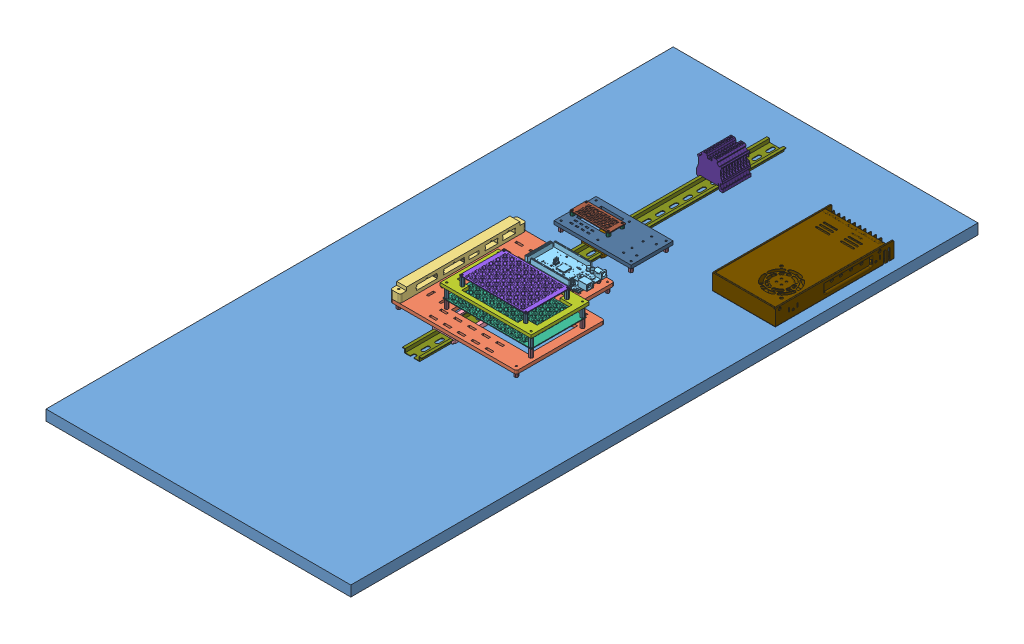
SolidWorks assembly Integrated Stand Base, configuration Default. Lengths in mm.
Overall size (552.45 92.11 1136.74).
89 component instances, 18 part files, 7 mates.
Components (placement in the parent):
- Base Stand-1: Base Stand [Default] at origin size (552.45 19.05 1136.74)
- Final_Assembly-1: Final_Assembly [Default] at (-199.0521 -63.7075 69.9554) x (0 0 -1) z (1 0 0) size (660.4 81.74 228.6)
  - Main board-1: Main board [Default] at (85.8748 92.7975 191.1146) size (228.6 6.1 228.6)
  - Connector_Holder-1: Connector_Holder [Default] at (-28.4252 98.8935 94.5946) size (228.6 20.32 17.78)
  - Main board din_rail-1: Main board din_rail [Default] at (200.1748 82.6375 173.6146) x (0 0 1) z (-1 0 0) size (40.89 10.16 228.6)
  - arduinoMega-1: arduinoMega [Detailed] at (160.8248 113.9303 205.0746) x (0 0 -1) z (1 0 0) size (108.32 14.5 53.3)
  - Flipper board-1: Flipper board [Default] at (53.4898 115.2003 220.1722) x (0 0 -1) z (-1 0 0) size (160.02 1.27 99.82)
  - LED_mount-1: LED_mount [Default] at (53.3628 133.7169 220.4262) x (0 0 -1) z (1 0 0) size (165.1 5.59 105.16)
  - LED_control_board-1: LED_control_board [Default] at (53.999 155.8149 220.1956) x (-0.002965 0 0.999996) z (0.999996 0 0.002965) size (120 1.47 80)
  - Output board din rail-1: Output board din rail [Default] at (241.4498 82.6375 173.6146) x (0 0 -1) z (1 0 0) size (40.89 10.16 76.2)
  - Output board-1: Output board [Default] at (317.6498 92.7975 243.4646) x (0 0 -1) z (1 0 0) size (139.7 6.1 76.2)
  - Output_Board-1: Output_Board [Default] at (279.9067 104.9133 144.6875) x (0 0 -1) z (1 0 0) size (71 1.47 30)
  - Spacer_Nut-3: Spacer_Nut [Default] at (6.8808 92.9245 296.8802) x (0 0 -1) z (0 1 0) size (6.48 5.61 2.41)
  - Spacer_Nut-5: Spacer_Nut [Default] at (6.8808 92.9245 143.769) x (0 0 -1) z (0 1 0) size (6.48 5.61 2.41)
  - Spacer_Nut-9: Spacer_Nut [Default] at (136.6748 92.9245 164.4446) x (0 0 -1) z (0 1 0) size (6.48 5.61 2.41)
  - Spacer_Nut-10: Spacer_Nut [Default] at (99.8448 92.9245 143.769) x (0 0 -1) z (0 1 0) size (6.48 5.61 2.41)
  - Spacer_Nut-12: Spacer_Nut [Default] at (136.6748 92.9245 239.1206) x (0.866025 0 -0.5) z (0 1 0) size (6.48 5.61 2.41)
  - Spacer_Nut-13: Spacer_Nut [Default] at (99.8448 92.9245 296.8802) x (0 0 -1) z (0 1 0) size (6.48 5.61 2.41)
  - Spacer_Nut-14: Spacer_Nut [Default] at (184.9348 92.9245 240.6446) x (0 0 -1) z (0 1 0) size (6.48 5.61 2.41)
  - Spacer_Nut-15: Spacer_Nut [Default] at (184.9348 92.9245 158.0946) x (0 0 -1) z (0 1 0) size (6.48 5.61 2.41)
  - Spacer_.592-1: Spacer_.592 [Default] at (6.8808 98.8935 143.769) x (0.866025 0 -0.5) z (0.5 0 0.866025) size (6.48 21.26 5.61)
  - Spacer_.592-2: Spacer_.592 [Default] at (6.8808 98.8935 296.8802) x (0 0 1) z (-1 0 0) size (6.48 21.26 5.61)
  - Spacer_.592-3: Spacer_.592 [Default] at (99.8448 98.8935 296.8802) x (0.866025 0 -0.5) z (0.5 0 0.866025) size (6.48 21.26 5.61)
  - Spacer_.592-4: Spacer_.592 [Default] at (99.8448 98.8935 143.769) x (0.866025 0 0.5) z (-0.5 0 0.866025) size (6.48 21.26 5.61)
  - Spacer_.592-5: Spacer_.592 [Default] at (136.6748 98.8935 164.4446) x (0.866025 0 -0.5) z (0.5 0 0.866025) size (6.48 21.26 5.61)
  - Spacer_.592-6: Spacer_.592 [Default] at (136.6748 98.8935 239.1206) x (0.866025 0 -0.5) z (0.5 0 0.866025) size (6.48 21.26 5.61)
  - Spacer_.592-7: Spacer_.592 [Default] at (184.9348 98.8935 240.6446) x (0.866025 0 -0.5) z (0.5 0 0.866025) size (6.48 21.26 5.61)
  - Spacer_.592-8: Spacer_.592 [Default] at (184.9348 98.8935 158.0946) x (0.866025 0 -0.5) z (0.5 0 0.866025) size (6.48 21.26 5.61)
  - Spacer_.778-6: Spacer_.778 [Default] at (6.8808 115.2003 296.8802) x (0.866025 0 0.5) z (-0.5 0 0.866025) size (6.48 21.26 5.61)
  - Spacer_.778-7: Spacer_.778 [Default] at (6.8808 115.2003 143.769) x (0 0 1) z (-1 0 0) size (6.48 21.26 5.61)
  - Spacer_.778-8: Spacer_.778 [Default] at (99.8448 115.2003 143.769) x (0.866025 0 0.5) z (-0.5 0 0.866025) size (6.48 21.26 5.61)
  - Spacer_.778-9: Spacer_.778 [Default] at (99.8448 115.2003 296.8802) x (0.866025 0 0.5) z (-0.5 0 0.866025) size (6.48 21.26 5.61)
  - Spacer_..237-2: Spacer_..237 [Default] at (6.8808 130.2371 296.8802) x (0.866025 0 -0.5) z (0.5 0 0.866025) size (6.48 12.24 5.61)
  - Spacer_..237-3: Spacer_..237 [Default] at (99.8448 130.2371 296.8802) x (0.866025 0 0.5) z (-0.5 0 0.866025) size (6.48 12.24 5.61)
  - Spacer_..237-4: Spacer_..237 [Default] at (6.8808 130.2371 143.769) x (0.866025 0 -0.5) z (0.5 0 0.866025) size (6.48 12.24 5.61)
  - Spacer_..237-5: Spacer_..237 [Default] at (99.8448 130.2371 143.769) x (0.866025 0 0.5) z (-0.5 0 0.866025) size (6.48 12.24 5.61)
  - Spacer_Nut-17: Spacer_Nut [Default] at (16.0248 133.8439 277.8862) x (0 0 -1) z (0 1 0) size (6.48 5.61 2.41)
  - Spacer_Nut-18: Spacer_Nut [Default] at (90.7008 133.8439 277.8862) x (-0.866025 0 -0.5) z (0 1 0) size (6.48 5.61 2.41)
  - Spacer_Nut-19: Spacer_Nut [Default] at (90.7008 133.8439 162.9662) x (0 0 -1) z (0 1 0) size (6.48 5.61 2.41)
  - Spacer_Nut-20: Spacer_Nut [Default] at (16.0248 133.8439 162.9662) x (-0.866025 0 0.5) z (0 1 0) size (6.48 5.61 2.41)
  - Spacer_.778-10: Spacer_.778 [Default] at (90.7008 139.3049 277.8862) x (0 0 1) z (-1 0 0) size (6.48 21.26 5.61)
  - Spacer_.778-11: Spacer_.778 [Default] at (90.7008 139.3049 162.9662) x (0.866025 0 -0.5) z (0.5 0 0.866025) size (6.48 21.26 5.61)
  - Spacer_.778-12: Spacer_.778 [Default] at (16.0248 139.3049 277.8862) x (0.866025 0 0.5) z (-0.5 0 0.866025) size (6.48 21.26 5.61)
  - Spacer_.778-13: Spacer_.778 [Default] at (16.0248 139.3049 162.9662) x (0.866025 0 -0.5) z (0.5 0 0.866025) size (6.48 21.26 5.61)
  - Spacer_..237-6: Spacer_..237 [Default] at (267.1038 98.8935 176.6626) x (0.5 0 0.866025) z (-0.866025 0 0.5) size (6.48 12.24 5.61)
  - 1.00m DIN Rail-1: 1.00m DIN Rail [26" LNG] at (414.4248 82.7575 173.6146) size (660.4 7.5 35)
  - Terminal Block Assembly-1: Terminal Block Assembly [Default] at (453.4648 83.4075 197.6146) x (1 0 0) z (0 1 0) size (51.51 55.11 56.59)
    - Terminal Block-2: Terminal Block [Default] at origin size (5.15 55.11 56.59)
      - pxc_3045088_17_UT-2-5-BK_3D.stp-1: pxc_3045088_17_UT-2-5-BK_3D.stp [Default] at origin size (5.15 55.11 56.59)
        - UT_2.5_BK-select.stp-1: UT_2.5_BK-select.stp [Default] at (5.15 -7.1989 17.4678) x (0 0.992546 -0.121869) z (1 0 0) size (49.27 50.96 5.15)
    - Terminal Block-3: Terminal Block [Default] at (5.1511 0 0) size (5.15 55.11 56.59)
      - pxc_3045088_17_UT-2-5-BK_3D.stp-1: pxc_3045088_17_UT-2-5-BK_3D.stp [Default] at origin size (5.15 55.11 56.59)
        - UT_2.5_BK-select.stp-1: UT_2.5_BK-select.stp [Default] at (5.15 -7.1989 17.4678) x (0 0.992546 -0.121869) z (1 0 0) size (49.27 50.96 5.15)
    - Terminal Block-4: Terminal Block [Default] at (10.3022 0 0) size (5.15 55.11 56.59)
      - pxc_3045088_17_UT-2-5-BK_3D.stp-1: pxc_3045088_17_UT-2-5-BK_3D.stp [Default] at origin size (5.15 55.11 56.59)
        - UT_2.5_BK-select.stp-1: UT_2.5_BK-select.stp [Default] at (5.15 -7.1989 17.4678) x (0 0.992546 -0.121869) z (1 0 0) size (49.27 50.96 5.15)
    - Terminal Block-5: Terminal Block [Default] at (15.4534 0 0) size (5.15 55.11 56.59)
      - pxc_3045088_17_UT-2-5-BK_3D.stp-1: pxc_3045088_17_UT-2-5-BK_3D.stp [Default] at origin size (5.15 55.11 56.59)
        - UT_2.5_BK-select.stp-1: UT_2.5_BK-select.stp [Default] at (5.15 -7.1989 17.4678) x (0 0.992546 -0.121869) z (1 0 0) size (49.27 50.96 5.15)
    - Terminal Block-6: Terminal Block [Default] at (20.6045 0 0) size (5.15 55.11 56.59)
      - pxc_3045088_17_UT-2-5-BK_3D.stp-1: pxc_3045088_17_UT-2-5-BK_3D.stp [Default] at origin size (5.15 55.11 56.59)
        - UT_2.5_BK-select.stp-1: UT_2.5_BK-select.stp [Default] at (5.15 -7.1989 17.4678) x (0 0.992546 -0.121869) z (1 0 0) size (49.27 50.96 5.15)
    - Terminal Block-7: Terminal Block [Default] at (25.7556 0 0) size (5.15 55.11 56.59)
      - pxc_3045088_17_UT-2-5-BK_3D.stp-1: pxc_3045088_17_UT-2-5-BK_3D.stp [Default] at origin size (5.15 55.11 56.59)
        - UT_2.5_BK-select.stp-1: UT_2.5_BK-select.stp [Default] at (5.15 -7.1989 17.4678) x (0 0.992546 -0.121869) z (1 0 0) size (49.27 50.96 5.15)
    - Terminal Block-8: Terminal Block [Default] at (30.9067 0 0) size (5.15 55.11 56.59)
      - pxc_3045088_17_UT-2-5-BK_3D.stp-1: pxc_3045088_17_UT-2-5-BK_3D.stp [Default] at origin size (5.15 55.11 56.59)
        - UT_2.5_BK-select.stp-1: UT_2.5_BK-select.stp [Default] at (5.15 -7.1989 17.4678) x (0 0.992546 -0.121869) z (1 0 0) size (49.27 50.96 5.15)
    - Terminal Block-9: Terminal Block [Default] at (36.0578 0 0) size (5.15 55.11 56.59)
      - pxc_3045088_17_UT-2-5-BK_3D.stp-1: pxc_3045088_17_UT-2-5-BK_3D.stp [Default] at origin size (5.15 55.11 56.59)
        - UT_2.5_BK-select.stp-1: UT_2.5_BK-select.stp [Default] at (5.15 -7.1989 17.4678) x (0 0.992546 -0.121869) z (1 0 0) size (49.27 50.96 5.15)
    - Terminal Block-10: Terminal Block [Default] at (41.209 0 0) size (5.15 55.11 56.59)
      - pxc_3045088_17_UT-2-5-BK_3D.stp-1: pxc_3045088_17_UT-2-5-BK_3D.stp [Default] at origin size (5.15 55.11 56.59)
        - UT_2.5_BK-select.stp-1: UT_2.5_BK-select.stp [Default] at (5.15 -7.1989 17.4678) x (0 0.992546 -0.121869) z (1 0 0) size (49.27 50.96 5.15)
    - Terminal Block-11: Terminal Block [Default] at (46.3601 0 0) size (5.15 55.11 56.59)
      - pxc_3045088_17_UT-2-5-BK_3D.stp-1: pxc_3045088_17_UT-2-5-BK_3D.stp [Default] at origin size (5.15 55.11 56.59)
        - UT_2.5_BK-select.stp-1: UT_2.5_BK-select.stp [Default] at (5.15 -7.1989 17.4678) x (0 0.992546 -0.121869) z (1 0 0) size (49.27 50.96 5.15)
  - Spacer_..237-7: Spacer_..237 [Default] at (291.9958 98.8935 176.6626) x (0.5 0 0.866025) z (-0.866025 0 0.5) size (6.48 12.24 5.61)
  - Spacer_..237-8: Spacer_..237 [Default] at (291.9958 98.8935 111.3846) x (0.5 0 0.866025) z (-0.866025 0 0.5) size (6.48 12.24 5.61)
  - Spacer_..237-9: Spacer_..237 [Default] at (267.1038 98.8935 111.3846) x (0.5 0 0.866025) z (-0.866025 0 0.5) size (6.48 12.24 5.61)
  - Spacer_.592-9: Spacer_.592 [Default] at (-20.8052 80.3007 84.4346) x (0 0 -1) z (1 0 0) size (6.48 21.26 5.61)
  - Spacer_.592-10: Spacer_.592 [Default] at (-20.8052 80.3007 297.7946) x (0 0 -1) z (1 0 0) size (6.48 21.26 5.61)
  - Spacer_.592-11: Spacer_.592 [Default] at (192.5548 80.3007 84.4346) x (0 0 -1) z (1 0 0) size (6.48 21.26 5.61)
  - Spacer_.592-12: Spacer_.592 [Default] at (193.8248 80.3007 248.2646) x (0 0 -1) z (1 0 0) size (6.48 21.26 5.61)
  - Spacer_.592-13: Spacer_.592 [Default] at (247.7998 80.3007 237.1146) x (0 0 -1) z (1 0 0) size (6.48 21.26 5.61)
  - Spacer_.592-14: Spacer_.592 [Default] at (311.2998 80.3007 237.1146) x (0 0 -1) z (1 0 0) size (6.48 21.26 5.61)
  - Spacer_.592-15: Spacer_.592 [Default] at (247.7998 80.3007 110.1146) x (0 0 -1) z (1 0 0) size (6.48 21.26 5.61)
  - Spacer_.592-16: Spacer_.592 [Default] at (311.2998 80.3007 110.1146) x (0 0 -1) z (1 0 0) size (6.48 21.26 5.61)
- Meanwell LRS-350-48 AC-DC Converter-1: Meanwell LRS-350-48 AC-DC Converter [Default] at (257.175 19.05 -220.0195) x (0 0 1) z (-1 0 0) size (215.21 30.1 114.01)
Mates (geometry in assembly coordinates):
- Parallel1: parallel aligned: plane of Base Stand-1 through (-276.225 19.05 568.3695) normal (0 0 1); plane of Final_Assembly-1/Main board-1 through (-122.2375 35.186 98.3805) normal (0 0 1)
- Distance1: distance = 153.9875 mm aligned: plane of Final_Assembly-1/Connector_Holder-1 through (-122.2375 35.186 98.3805) normal (-1 0 0); plane of Base Stand-1 through (-276.225 19.05 568.3695) normal (-1 0 0)
- Distance2: distance = 63.5 mm aligned: plane of Final_Assembly-1/1.00m DIN Rail-1 through (-7.9375 19.05 -504.8695) normal (0 0 -1); plane of Base Stand-1 through (-276.225 19.05 -568.3695) normal (0 0 -1)
- Coincident5: coincident anti-aligned: plane of Base Stand-1 through (0 19.05 0) normal (0 1 0); plane of Final_Assembly-1/1.00m DIN Rail-1 through (-7.9375 19.05 155.5305) normal (0 -1 0)
- Distance3: distance = 19.05 mm aligned: plane of Meanwell LRS-350-48 AC-DC Converter-1 through (257.175 69.05 -435.0194) normal (1 0 0); plane of Base Stand-1 through (276.225 19.05 568.3695) normal (1 0 0)
- Coincident7: coincident anti-aligned: plane of Base Stand-1 through (0 19.05 0) normal (0 1 0); plane of Meanwell LRS-350-48 AC-DC Converter-1 through (257.175 19.05 -435.0194) normal (0 -1 0)
- Distance4: distance = 133.35 mm aligned: plane of Meanwell LRS-350-48 AC-DC Converter-1 through (143.175 19.05 -435.0194) normal (0 0 -1); plane of Base Stand-1 through (-276.225 19.05 -568.3695) normal (0 0 -1)
